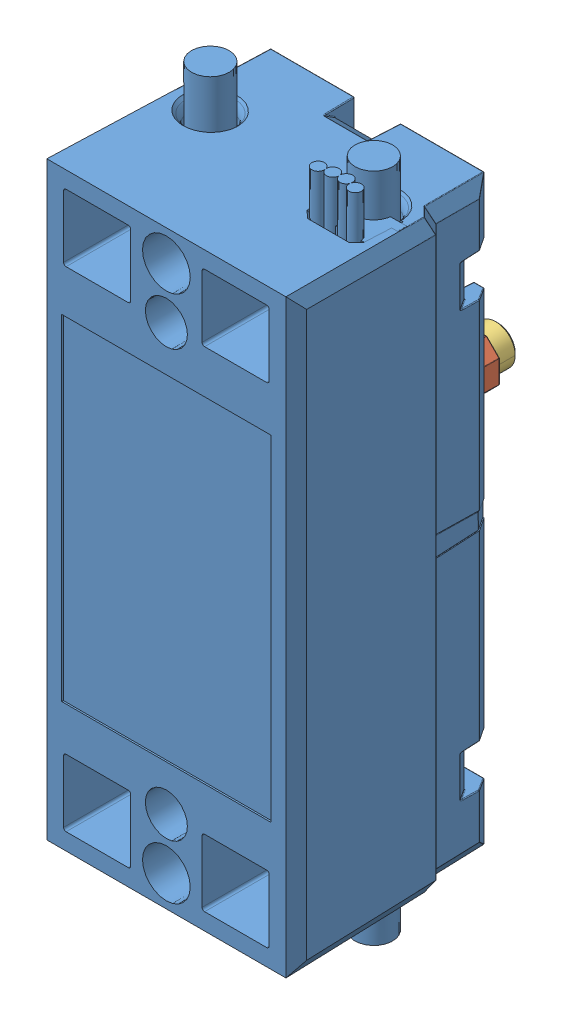
SolidWorks assembly Talon_SRX_217-8080_No_Wires, configuration Default. Lengths in mm.
Overall size (30.47 80 30.05).
5 component instances, 3 part files, 0 mates.
Components (placement in the parent):
- Talon_SRX_217-8080_No_Wires.STEP-1: Talon_SRX_217-8080_No_Wires.STEP [Default] at origin size (30.47 80 30.05)
  - 217-8080-baseRev4_no wires.STEP-1: 217-8080-baseRev4_no wires.STEP [Default] at origin size (30.47 80 25.2)
  - 217-8080-002 Rev1.STEP-1: 217-8080-002 Rev1.STEP [Default] at (0 13.05 -9.65) x (1 0 0) z (0 -1 0) size (25.15 2.9 7.5)
  - 217-8080-005 Rev1_91251A105.STEP-1: 217-8080-005 Rev1_91251A105.STEP [Default] at (-9.525 13.05 -5.8875) size (4.65 4.65 7.61)
  - 217-8080-005 Rev1_91251A105.STEP-2: 217-8080-005 Rev1_91251A105.STEP [Default] at (9.525 13.05 -5.8875) size (4.65 4.65 7.61)
